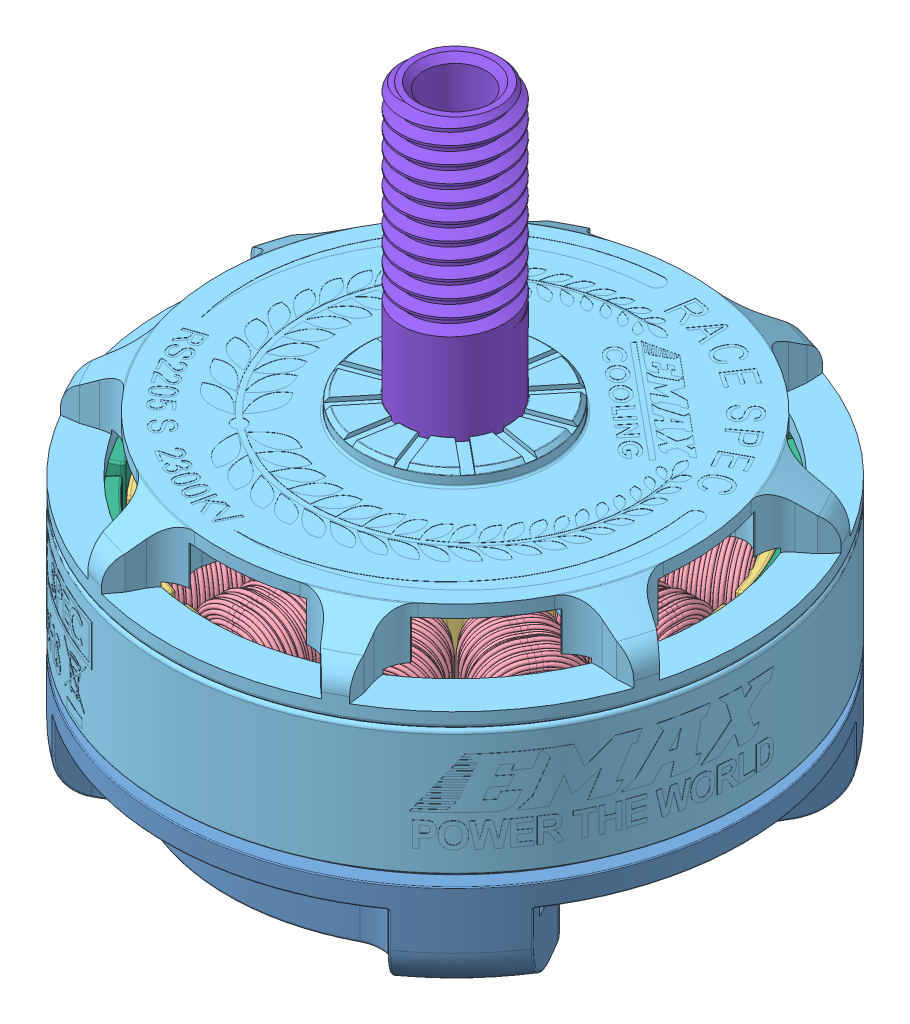
SolidWorks assembly EMAX RS2205S, configuration Predeterminado. Lengths in mm.
Overall size (39.3 30.6 39.3).
24 component instances, 10 part files, 11 mates.
Components (placement in the parent):
- STATOR-1: STATOR [Predeterminado] at origin size (27.9 11.97 27.9)
  - STATOR-1: STATOR [Predeterminado] at origin size (27.9 10.76 27.9)
  - BEARING-1: BEARING [Predeterminado] at (0 1.95 0) x (1 0 0) z (0 1 0) size (8 8 3.5)
  - BEARING-2: BEARING [Predeterminado] at (0 8.85 0) x (-0.982082 0 -0.188455) z (0 -1 0) size (8 8 3.5)
  - STATOR SLEEVE-1: STATOR SLEEVE [Predeterminado] at (0 5.25 0) size (22.5 5.67 22.5)
  - WINDING-1: WINDING [Predeterminado] at (8.4112 8.075 0) size (4.68 7.47 4.47)
  - WINDING-2: WINDING [Predeterminado] at (7.2843 8.075 4.2056) x (0.866025 0 0.5) z (-0.5 0 0.866025) size (4.68 7.47 4.47)
  - WINDING-3: WINDING [Predeterminado] at (4.2056 8.075 7.2843) x (0.5 0 0.866025) z (-0.866025 0 0.5) size (4.68 7.47 4.47)
  - WINDING-4: WINDING [Predeterminado] at (0 8.075 8.4112) x (0 0 1) z (-1 0 0) size (4.68 7.47 4.47)
  - WINDING-5: WINDING [Predeterminado] at (-4.2056 8.075 7.2843) x (-0.5 0 0.866025) z (-0.866025 0 -0.5) size (4.68 7.47 4.47)
  - WINDING-6: WINDING [Predeterminado] at (-7.2843 8.075 4.2056) x (-0.866025 0 0.5) z (-0.5 0 -0.866025) size (4.68 7.47 4.47)
  - WINDING-7: WINDING [Predeterminado] at (-8.4112 8.075 0) x (-1 0 0) z (0 0 -1) size (4.68 7.47 4.47)
  - WINDING-8: WINDING [Predeterminado] at (-7.2843 8.075 -4.2056) x (-0.866025 0 -0.5) z (0.5 0 -0.866025) size (4.68 7.47 4.47)
  - WINDING-9: WINDING [Predeterminado] at (-4.2056 8.075 -7.2843) x (-0.5 0 -0.866025) z (0.866025 0 -0.5) size (4.68 7.47 4.47)
  - WINDING-10: WINDING [Predeterminado] at (0 8.075 -8.4112) x (0 0 -1) z (1 0 0) size (4.68 7.47 4.47)
  - WINDING-11: WINDING [Predeterminado] at (4.2056 8.075 -7.2843) x (0.5 0 -0.866025) z (0.866025 0 0.5) size (4.68 7.47 4.47)
  - WINDING-12: WINDING [Predeterminado] at (7.2843 8.075 -4.2056) x (0.866025 0 -0.5) z (0.5 0 0.866025) size (4.68 7.47 4.47)
- ROTOR-1: ROTOR [Predeterminado] at (0 0.05 0) x (0.771425 0 0.636321) z (-0.636321 0 0.771425) size (27.91 28.74 27.91)
  - ROTOR BELL-1: ROTOR BELL [Predeterminado] at origin size (27.91 10.2 27.91)
  - MAGNETS-1: MAGNETS [Predeterminado] at (0 5.3 0) size (25.73 6 25.8)
  - MAGNETS ADHESIVE-1: MAGNETS ADHESIVE [Predeterminado] at (0 5.4 0) size (26 5.9 26)
  - SHAFT-1: SHAFT [Predeterminado] at (0 0.2 0) size (7.2 28.74 7.2)
- WASHER-1: WASHER [Predeterminado] at (0 -0.6 0) x (0.636321 0 -0.771425) z (0.771425 0 0.636321) size (5 0.8 5)
- SCREW-3: SCREW [ROSCADO] at (0 3.4 0) x (0 1 0) z (-0.946141 0 -0.323755) size (5.25 3.8 3.8)
Mates (geometry in assembly coordinates):
- Coincidente1: coincident aligned: plane of STATOR-1/STATOR-1 through (0 0 0) normal (0 0 1); plane of assembly through (0 0 0) normal (0 0 1)
- Coincidente2: coincident anti-aligned: plane of STATOR-1/STATOR-1 through (-11.95 0 0) normal (0 -1 0); plane of assembly through (0 0 0) normal (0 1 0)
- Coincidente3: coincident aligned: plane of STATOR-1/STATOR-1 through (0 0 0) normal (1 0 0); plane of assembly through (0 0 0) normal (1 0 0)
- Concéntrica1: concentric aligned: cylinder of STATOR-1/STATOR-1 through (0 0 0) axis (0 -1 0) radius 13.95; cylinder of ROTOR-1/ROTOR BELL-1 through (0 0.05 0) axis (0 -1 0) radius 13.95
- Coincidente6: coincident anti-aligned: plane of STATOR-1/BEARING-2 through (0.3644 10.6 -1.8989) normal (0 1 0); plane of ROTOR-1/SHAFT-1 through (2.2371 10.6 1.8453) normal (0 -1 0)
- Concéntrica2: concentric aligned: cylinder of ROTOR-1/SHAFT-1 through (0 0.25 0) axis (0 -1 0) radius 0.8; cylinder of WASHER-1 through (0 0.2 0) axis (0 -1 0) radius 1.1
- Concéntrica41: concentric aligned: cone of WASHER-1 through (0 -0.6 0) axis (0 1 0); cylinder of SCREW-3 through (0 3.4 0) axis (0 1 0) radius 1.9
- Coincidente91: coincident anti-aligned: plane of WASHER-1 through (0 -0.6 0) normal (0 -1 0); plane of SCREW-3 through (0.3561 -0.6 -1.0408) normal (0 1 0)
- Bloquear1: lock: unknown of ?; unknown of SCREW-3
- Bloquear2: lock: unknown of ?; unknown of WASHER-1
- Coincidente93: coincident anti-aligned: plane of STATOR-1/BEARING-1 through (0 0.2 -1.9336) normal (0 -1 0); plane of WASHER-1 through (0 0.2 0) normal (0 1 0)
